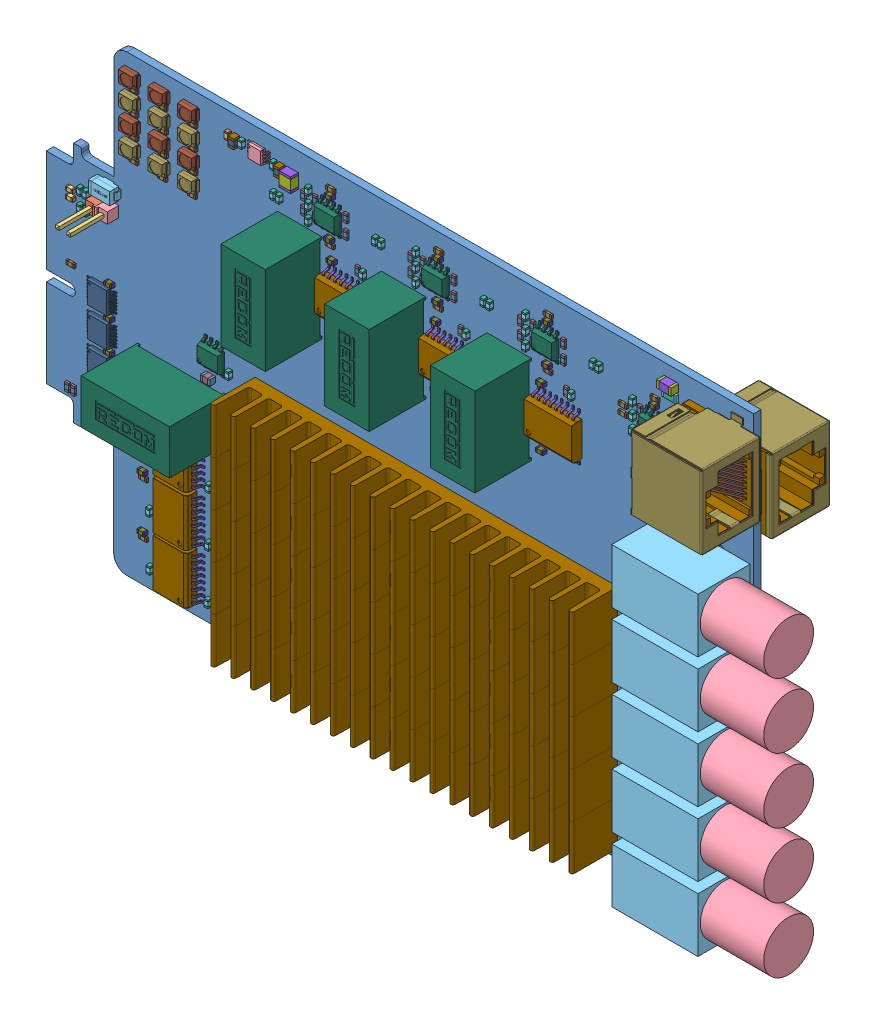
SolidWorks assembly 1166V10, configuration Standard. Lengths in mm. (continued)
Components (placement in the parent): (continued)
- 1166V10.step-1: 1166V10.step [Standard] at origin size (170.01 100 28.53) (continued)
  - C206.step-1: C206.step [Standard] at origin size (5.7 5 2.5) (continued)
    - 6545673728.step-2: 6545673728.step [Standard] at (105.025 49.3 -4.122) size (0.65 5 2.5)
      - Extruded-32.step-1: Extruded-32.step [Standard] at origin size (0.65 5 2.5)
    - 6545673168.step-1: 6545673168.step [Standard] at (107.55 49.3 -4.122) size (4.4 5 2.5)
      - Extruded-31.step-1: Extruded-31.step [Standard] at origin size (4.4 5 2.5)
  - C205.step-1: C205.step [Standard] at origin size (5.7 5 2.5)
    - 6545673728.step-1: 6545673728.step [Standard] at (110.075 43.2 -4.122) size (0.65 5 2.5)
      - Extruded-32.step-1: Extruded-32.step [Standard] at origin size (0.65 5 2.5)
    - 6545673728.step-2: 6545673728.step [Standard] at (105.025 43.2 -4.122) size (0.65 5 2.5)
      - Extruded-32.step-1: Extruded-32.step [Standard] at origin size (0.65 5 2.5)
    - 6545673168.step-1: 6545673168.step [Standard] at (107.55 43.2 -4.122) size (4.4 5 2.5)
      - Extruded-31.step-1: Extruded-31.step [Standard] at origin size (4.4 5 2.5)
  - C204.step-1: C204.step [Standard] at origin size (5.7 5 2.5)
    - 6545673728.step-1: 6545673728.step [Standard] at (117.625 43.2 -4.122) size (0.65 5 2.5)
      - Extruded-32.step-1: Extruded-32.step [Standard] at origin size (0.65 5 2.5)
    - 6545673728.step-2: 6545673728.step [Standard] at (122.675 43.2 -4.122) size (0.65 5 2.5)
      - Extruded-32.step-1: Extruded-32.step [Standard] at origin size (0.65 5 2.5)
    - 6545673168.step-1: 6545673168.step [Standard] at (120.15 43.2 -4.122) size (4.4 5 2.5)
      - Extruded-31.step-1: Extruded-31.step [Standard] at origin size (4.4 5 2.5)
  - C104.step-1: C104.step [Standard] at origin size (0.82 1.6 0.9)
    - 6547668352.step-1: 6547668352.step [Standard] at (7.9 65.55 0) size (0.82 0.9 0.9)
      - Extruded.step-1: Extruded.step [Standard] at origin size (0.82 0.9 0.9)
    - 6549602528.step-1: 6549602528.step [Standard] at (7.9 66.175 0) size (0.82 0.35 0.9)
      - Extruded-0.step-1: Extruded-0.step [Standard] at origin size (0.82 0.35 0.9)
    - 6549602528.step-2: 6549602528.step [Standard] at (7.9 64.925 0) size (0.82 0.35 0.9)
      - Extruded-0.step-1: Extruded-0.step [Standard] at origin size (0.82 0.35 0.9)
  - C103.step-1: C103.step [Standard] at origin size (0.82 1.6 0.9)
    - 6547668352.step-1: 6547668352.step [Standard] at (9.2 65.55 0) size (0.82 0.9 0.9)
      - Extruded.step-1: Extruded.step [Standard] at origin size (0.82 0.9 0.9)
    - 6549602528.step-1: 6549602528.step [Standard] at (9.2 66.175 0) size (0.82 0.35 0.9)
      - Extruded-0.step-1: Extruded-0.step [Standard] at origin size (0.82 0.35 0.9)
    - 6549602528.step-2: 6549602528.step [Standard] at (9.2 64.925 0) size (0.82 0.35 0.9)
      - Extruded-0.step-1: Extruded-0.step [Standard] at origin size (0.82 0.35 0.9)
  - Free-Models.step-1: Free-Models.step [Standard] at origin size (80 50 10)
    - sk545_-_80x50x10mm.step-1: sk545_-_80x50x10mm.step [Standard] at (47 13 1) x (1 0 0) z (0 -1 0) size (80 10 10)
    - sk545_-_80x50x10mm.step-2: sk545_-_80x50x10mm.step [Standard] at (47 23 1) x (1 0 0) z (0 -1 0) size (80 10 10)
    - sk545_-_80x50x10mm.step-3: sk545_-_80x50x10mm.step [Standard] at (47 33 1) x (1 0 0) z (0 -1 0) size (80 10 10)
    - sk545_-_80x50x10mm.step-4: sk545_-_80x50x10mm.step [Standard] at (47 43 1) x (1 0 0) z (0 -1 0) size (80 10 10)
    - sk545_-_80x50x10mm.step-5: sk545_-_80x50x10mm.step [Standard] at (47 53 1) x (1 0 0) z (0 -1 0) size (80 10 10)
